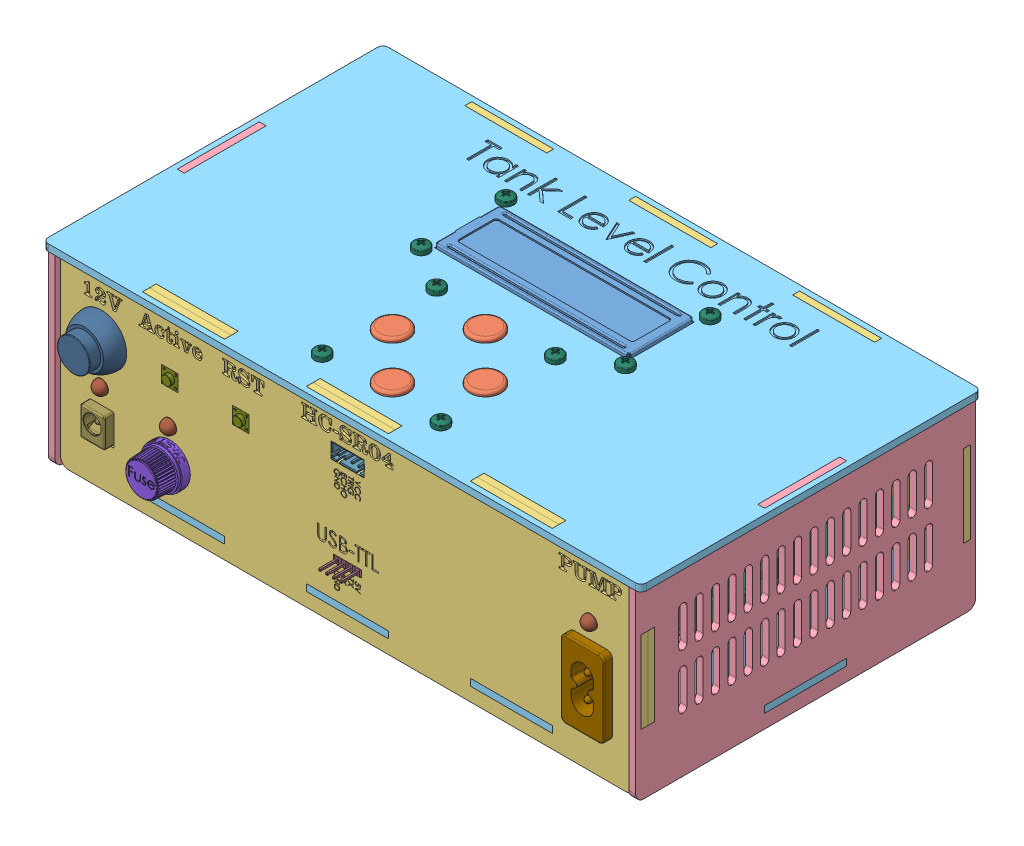
SolidWorks assembly assembly, configuration Default. Lengths in mm.
Overall size (219 72.37 133).
31 component instances, 16 part files, 51 mates.
Components (placement in the parent):
- DFRobot_1602_LCD-2: DFRobot_1602_LCD [Default] at (80.4235 150.9642 122.8308) size (80 10.64 36)
- arrowsKeypad-2: arrowsKeypad [Default] at (137.7127 144.1083 69.6587) x (-1 0 0) z (0 1 0) size (64.42 48.64 13.05)
- boxAssembly-1: boxAssembly [Default] at (-5.2675 50.6588 14.6624) size (219 70 124.5)
  - boxFront-2: boxFront [Side] at (84.1854 69.861 71.9101) size (215 70 2.5)
  - boxSide-1: boxSide [Default] at (-22.0646 69.861 130.9101) size (2.5 70 124.5)
  - boxSide-2: boxSide [Default] at (190.4354 69.861 130.9101) size (2.5 70 124.5)
  - boxTop-1: boxTop [Default] at (84.1854 101.111 130.9101) size (219 2.5 124.5)
  - boxTop-2: boxTop [Bottom] at (84.1854 38.611 130.9101) size (215 2.5 120.5)
  - boxFront-3: boxFront [Front] at (84.1854 69.861 189.9101) size (215 70 2.5)
  - boxFront-4: boxFront [Middle] at (84.1854 69.861 187.4101) size (215 70 2.5)
- controlCircuit-2: controlCircuit [Default] at (14.7389 110.5198 218.2665) x (1 0 0) z (0 1 0) size (140.72 109.59 35.62)
- powerCircuit-2: powerCircuit [Default] at (-153.7021 110.5198 205.3125) x (1 0 0) z (0 1 0) size (57.77 82.04 42.52)
- Fuse holder-1: Fuse holder [Default] at (13.9179 103.6248 215.8225) size (15 17.32 35.5)
- 771wx201-1: 771wx201 [Default] at (167.9179 110.5316 205.8225) x (0 -1 0) z (0 0 -1) size (28.55 16 22.5)
- MomentarySwitch-1: MomentarySwitch [Default] at (-11.0821 130.5198 182.8225) x (1 0 0) z (0 -1 0) size (18.4 38.3 18.4)
- LED 5mm-1: LED 5mm [Valor predeterminado] at (-11.0821 115.5198 199.8225) size (5.5 6 35.8)
- DC Power Jack 5.5mm x 2.1mm-2: DC Power Jack 5.5mm x 2.1mm [Default] at (-11.0821 105.1948 205.8225) size (9.77 14.38 14.62)
- LED 5mm-2: LED 5mm [Valor predeterminado] at (13.9179 115.5198 199.8225) size (5.5 6 35.8)
- LED 5mm-3: LED 5mm [Valor predeterminado] at (167.9179 130.5198 199.8225) size (5.5 6 35.8)
- Header male 4 pins-1: Header male 4 pins [Default] at (78.9179 103.6248 203.2225) x (1 0 0) z (0 -1 0) size (10.16 12.7 2.54)
- JST_B4B-1: JST_B4B [Default] at (79.0479 137.4198 198.8225) x (1 0 0) z (0 -1 0) size (12.4 10.4 5.75)
- pan cross head_am-2: pan cross head_am [B18.6.7M - M3 x 0.5 x 6 Type I Cross Recessed PHMS --6N] at (41.5479 155.4198 110.4125) x (0 -1 0) z (0 0 1) size (8.37 5.6 5.6)
- pan cross head_am-3: pan cross head_am [B18.6.7M - M3 x 0.5 x 6 Type I Cross Recessed PHMS --6N] at (116.2879 155.4198 110.4125) x (0 -1 0) z (0 0 1) size (8.37 5.6 5.6)
- pan cross head_am-4: pan cross head_am [B18.6.7M - M3 x 0.5 x 6 Type I Cross Recessed PHMS --6N] at (116.2879 155.4198 141.4125) x (0 -1 0) z (0 0 1) size (8.37 5.6 5.6)
- pan cross head_am-5: pan cross head_am [B18.6.7M - M3 x 0.5 x 6 Type I Cross Recessed PHMS --6N] at (41.5479 155.4198 141.4125) x (0 -1 0) z (0 0 1) size (8.37 5.6 5.6)
- pan cross head_am-6: pan cross head_am [B18.6.7M - M3 x 0.5 x 16 Type I Cross Recessed PHMS --16N] at (100.6574 155.4198 151.4125) x (0 -1 0) z (0 0 1) size (18.37 5.6 5.6)
- pan cross head_am-7: pan cross head_am [B18.6.7M - M3 x 0.5 x 16 Type I Cross Recessed PHMS --16N] at (57.1784 155.4198 151.4125) x (0 -1 0) z (0 0 1) size (18.37 5.6 5.6)
- pan cross head_am-9: pan cross head_am [B18.6.7M - M3 x 0.5 x 16 Type I Cross Recessed PHMS --16N] at (57.1784 155.4198 193.3225) x (0 -1 0) z (0 0 1) size (18.37 5.6 5.6)
- pan cross head_am-10: pan cross head_am [B18.6.7M - M3 x 0.5 x 16 Type I Cross Recessed PHMS --16N] at (100.6574 155.4198 193.3225) x (0 -1 0) z (0 0 1) size (18.37 5.6 5.6)
- Tactile switch 6x6x5mm-3: Tactile switch 6x6x5mm [Default] at (13.9229 130.5148 202.2125) x (1 0 0) z (0 -1 0) size (6.03 8.52 7.74)
- Tactile switch 6x6x5mm-2: Tactile switch 6x6x5mm [Default] at (39.9229 130.5148 202.2125) x (1 0 0) z (0 -1 0) size (6.03 8.52 7.74)
Mates (geometry in assembly coordinates):
- Distance1: distance = 20 mm: plane of boxAssembly-1/boxTop-2 through (78.9179 90.5198 145.5725) normal (0 1 0); plane of powerCircuit-2 through (-19.1301 110.5198 170.8165) normal (0 -1 0)
- Coincident3: coincident: plane of controlCircuit-2 through (14.7389 110.5198 218.2665) normal (0 -1 0); plane of powerCircuit-2 through (-19.1301 110.5198 170.8165) normal (0 -1 0)
- Coincident11: coincident: plane of boxAssembly-1/boxFront-3 through (78.9179 120.5198 205.8225) normal (0 0 1); plane of 771wx201-1 through (161.9179 98.4316 205.8225) normal (0 0 -1)
- Coincident16: coincident: plane of boxAssembly-1/boxFront-3 through (161.9179 98.1948 195.8225) normal (1 0 0); plane of 771wx201-1 through (161.9179 119.0316 193.3225) normal (-1 0 0)
- Coincident13: coincident: plane of boxAssembly-1/boxFront-3 through (78.9179 120.5198 205.8225) normal (0 0 1); plane of Fuse holder-1 through (13.9179 103.6248 205.8225) normal (0 0 -1)
- Coincident14: coincident: plane of boxAssembly-1/boxFront-3 through (78.9179 120.5198 205.8225) normal (0 0 1); plane of MomentarySwitch-1 through (-11.0821 130.5198 205.8225) normal (0 0 -1)
- Coincident15: coincident: plane of boxAssembly-1/boxFront-3 through (161.9179 122.1948 195.8225) normal (0 -1 0); plane of 771wx201-1 through (164.4179 122.1948 198.6117) normal (0 1 0)
- Concentric1: concentric: cylinder of boxAssembly-1/boxFront-3 through (-11.0821 130.5198 195.8225) axis (0 0 1) radius 5.85; cylinder of MomentarySwitch-1 through (-11.0821 130.5198 205.8225) axis (0 0 -1) radius 5
- Concentric2: concentric: cylinder of boxAssembly-1/boxFront-3 through (13.9179 103.6248 195.8225) axis (0 0 1) radius 6; cylinder of Fuse holder-1 through (13.9179 103.6248 196.8225) axis (0 0 -1) radius 4
- Concentric4: concentric: cylinder of boxAssembly-1/boxFront-3 through (-11.0821 115.5198 195.8225) axis (0 0 1) radius 2.5; cylinder of LED 5mm-1 through (-11.0821 115.5198 200.8225) axis (0 0 -1) radius 2.5
- Coincident18: coincident: plane of boxAssembly-1/boxFront-4 through (78.9179 120.5198 200.8225) normal (0 0 -1); plane of LED 5mm-1 through (-11.0821 115.5198 200.8225) normal (0 0 1)
- Coincident20: coincident: plane of boxAssembly-1/boxFront-3 through (78.9179 120.5198 205.8225) normal (0 0 1); plane of DC Power Jack 5.5mm x 2.1mm-2 through (-11.0821 105.1948 205.8225) normal (0 0 -1)
- Concentric5: concentric: cylinder of boxAssembly-1/boxFront-3 through (-11.0821 105.1948 195.8225) axis (0 0 1) radius 3.86; cone of DC Power Jack 5.5mm x 2.1mm-2 through (-11.0821 105.1948 205.8225) axis (0 0 -1)
- Concentric6: concentric: cylinder of boxAssembly-1/boxFront-3 through (13.9179 115.5198 195.8225) axis (0 0 1) radius 2.5; cylinder of LED 5mm-2 through (13.9179 115.5198 200.8225) axis (0 0 -1) radius 2.5
- Concentric7: concentric: cylinder of boxAssembly-1/boxFront-3 through (167.9179 130.5198 195.8225) axis (0 0 1) radius 2.5; cylinder of LED 5mm-3 through (167.9179 130.5198 200.8225) axis (0 0 -1) radius 2.5
- Distance3: distance = 3 mm: plane of boxAssembly-1/boxTop-1 through (78.9179 150.5198 145.5725) normal (0 -1 0); plane of DFRobot_1602_LCD-2 through (79.0179 147.5198 125.9125) normal (0 1 0)
- Coincident27: coincident: plane of boxAssembly-1/boxTop-1 through (43.3179 143.0198 114.4125) normal (0 0 1); plane of DFRobot_1602_LCD-2 through (113.6679 149.5198 114.4125) normal (0 0 -1)
- Coincident28: coincident: plane of DFRobot_1602_LCD-2 through (114.5179 151.0198 137.5625) normal (1 0 0); plane of boxAssembly-1/boxTop-1 through (114.5179 143.0198 138.4125) normal (-1 0 0)
- Coincident29: coincident: plane of boxAssembly-1/boxFront-3 through (73.8379 102.3548 195.8225) normal (0 1 0); plane of Header male 4 pins-1 through (83.9979 102.3548 206.0225) normal (0 -1 0)
- Coincident30: coincident: plane of boxAssembly-1/boxFront-3 through (73.8379 102.3548 195.8225) normal (1 0 0); plane of Header male 4 pins-1 through (73.8379 103.6248 204.6225) normal (-1 0 0)
- Coincident32: coincident: plane of boxAssembly-1/boxFront-3 through (78.9179 120.5198 205.8225) normal (0 0 1); line of Header male 4 pins-1 through (81.1079 104.8948 205.8225) axis (-1 0 0)
- Concentric8: concentric: cylinder of boxAssembly-1/boxTop-1 through (41.5479 143.0198 110.4125) axis (0 1 0) radius 1.5; cylinder of pan cross head_am-2 through (41.5479 180.8198 110.4125) axis (0 1 0) radius 2.8
- Coincident33: coincident: plane of boxAssembly-1/boxTop-1 through (78.9179 153.0198 145.5725) normal (0 1 0); plane of pan cross head_am-2 through (43.0479 153.0198 110.4125) normal (0 -1 0)
- Concentric9: concentric: cylinder of boxAssembly-1/boxTop-1 through (116.2879 143.0198 110.4125) axis (0 1 0) radius 1.5; cylinder of pan cross head_am-3 through (116.2879 180.8198 110.4125) axis (0 1 0) radius 2.8
- Coincident34: coincident: plane of boxAssembly-1/boxTop-1 through (78.9179 153.0198 145.5725) normal (0 1 0); plane of pan cross head_am-3 through (117.7879 153.0198 110.4125) normal (0 -1 0)
- Concentric10: concentric: cylinder of boxAssembly-1/boxTop-1 through (116.2879 143.0198 141.4125) axis (0 1 0) radius 1.5; cylinder of pan cross head_am-4 through (116.2879 180.8198 141.4125) axis (0 1 0) radius 2.8
- Coincident35: coincident: plane of boxAssembly-1/boxTop-1 through (78.9179 153.0198 145.5725) normal (0 1 0); plane of pan cross head_am-4 through (117.7879 153.0198 141.4125) normal (0 -1 0)
- Concentric11: concentric: cylinder of boxAssembly-1/boxTop-1 through (41.5479 143.0198 141.4125) axis (0 1 0) radius 1.5; cylinder of pan cross head_am-5 through (41.5479 180.8198 141.4125) axis (0 1 0) radius 2.8
- Coincident36: coincident: plane of boxAssembly-1/boxTop-1 through (78.9179 153.0198 145.5725) normal (0 1 0); plane of pan cross head_am-5 through (43.0479 153.0198 141.4125) normal (0 -1 0)
- Coincident37: coincident: plane of boxAssembly-1/boxFront-3 through (72.8479 134.5448 195.8225) normal (0 1 0); plane of JST_B4B-1 through (82.7479 134.5448 205.8225) normal (0 -1 0)
- Coincident38: coincident: plane of boxAssembly-1/boxFront-3 through (72.8479 140.2948 195.8225) normal (1 0 0); plane of JST_B4B-1 through (72.8479 134.5448 205.8225) normal (-1 0 0)
- Coincident39: coincident: plane of boxAssembly-1/boxFront-3 through (78.9179 120.5198 205.8225) normal (0 0 1); plane of JST_B4B-1 through (77.7979 137.4198 205.8225) normal (0 0 1)
- Distance2: distance = 6 mm: plane of boxAssembly-1/boxTop-1 through (78.9179 150.5198 145.5725) normal (0 -1 0); plane of arrowsKeypad-2 through (137.7127 144.5198 69.6587) normal (0 1 0)
- Concentric151: concentric: cylinder of boxAssembly-1/boxTop-1 through (100.6574 143.0198 151.4125) axis (0 1 0) radius 1.5; cylinder of pan cross head_am-6 through (100.6574 180.8198 151.4125) axis (0 1 0) radius 2.8
- Coincident421: coincident: plane of boxAssembly-1/boxTop-1 through (78.9179 153.0198 145.5725) normal (0 1 0); plane of pan cross head_am-6 through (102.1574 153.0198 151.4125) normal (0 -1 0)
- Concentric161: concentric: cylinder of boxAssembly-1/boxTop-1 through (57.1784 143.0198 151.4125) axis (0 1 0) radius 1.5; cylinder of pan cross head_am-7 through (57.1784 180.8198 151.4125) axis (0 1 0) radius 2.8
- Coincident431: coincident: plane of boxAssembly-1/boxTop-1 through (78.9179 153.0198 145.5725) normal (0 1 0); plane of pan cross head_am-7 through (58.6784 153.0198 151.4125) normal (0 -1 0)
- Concentric171: concentric: cylinder of boxAssembly-1/boxTop-1 through (57.1784 143.0198 193.3225) axis (0 1 0) radius 1.5; cylinder of pan cross head_am-9 through (57.1784 180.8198 193.3225) axis (0 1 0) radius 2.8
- Coincident441: coincident: plane of boxAssembly-1/boxTop-1 through (78.9179 153.0198 145.5725) normal (0 1 0); plane of pan cross head_am-9 through (58.6784 153.0198 193.3225) normal (0 -1 0)
- Concentric181: concentric: cylinder of boxAssembly-1/boxTop-1 through (100.6574 143.0198 193.3225) axis (0 1 0) radius 1.5; cylinder of pan cross head_am-10 through (100.6574 180.8198 193.3225) axis (0 1 0) radius 2.8
- Coincident451: coincident: plane of boxAssembly-1/boxTop-1 through (78.9179 153.0198 145.5725) normal (0 1 0); plane of pan cross head_am-10 through (102.1574 153.0198 193.3225) normal (0 -1 0)
- Concentric182: concentric: cylinder of arrowsKeypad-2 through (78.9177 154.5198 155.3069) axis (0 -1 0) radius 5.75; cylinder of boxAssembly-1/boxTop-1 through (78.9177 153.0198 155.3069) axis (0 -1 0) radius 5.75
- Concentric183: concentric: cylinder of arrowsKeypad-2 through (95.9319 154.5198 172.3211) axis (0 -1 0) radius 5.75; cylinder of boxAssembly-1/boxTop-1 through (95.9319 153.0198 172.3211) axis (0 -1 0) radius 5.75
- Concentric184: concentric: circle of boxAssembly-1/boxTop-2; circle of controlCircuit-2
- Concentric185: concentric: circle of boxAssembly-1/boxTop-2; circle of powerCircuit-2
- Coincident452: coincident: plane of Tactile switch 6x6x5mm-3 through (11.2279 127.8198 205.8225) normal (0 0 1); plane of Tactile switch 6x6x5mm-2 through (37.2279 127.8198 205.8225) normal (0 0 1)
- Coincident453: coincident: plane of boxAssembly-1/boxFront-3 through (78.9179 120.5198 205.8225) normal (0 0 1); plane of Tactile switch 6x6x5mm-2 through (37.2279 127.8198 205.8225) normal (0 0 1)
- Coincident454: coincident: plane of boxAssembly-1/boxFront-3 through (42.9179 127.5198 195.8225) normal (-1 0 0); plane of Tactile switch 6x6x5mm-2 through (42.9179 133.2098 205.8225) normal (1 0 0)
- Coincident455: coincident: plane of Tactile switch 6x6x5mm-3 through (11.2279 127.5198 205.8225) normal (0 -1 0); plane of Tactile switch 6x6x5mm-2 through (37.2279 127.5198 205.8225) normal (0 -1 0)
- Coincident456: coincident: plane of boxAssembly-1/boxFront-3 through (36.9179 127.5198 195.8225) normal (0 1 0); plane of Tactile switch 6x6x5mm-2 through (37.2279 127.5198 205.8225) normal (0 -1 0)
- Coincident457: coincident: plane of boxAssembly-1/boxFront-3 through (16.9179 127.5198 195.8225) normal (-1 0 0); plane of Tactile switch 6x6x5mm-3 through (16.9179 133.2098 205.8225) normal (1 0 0)
